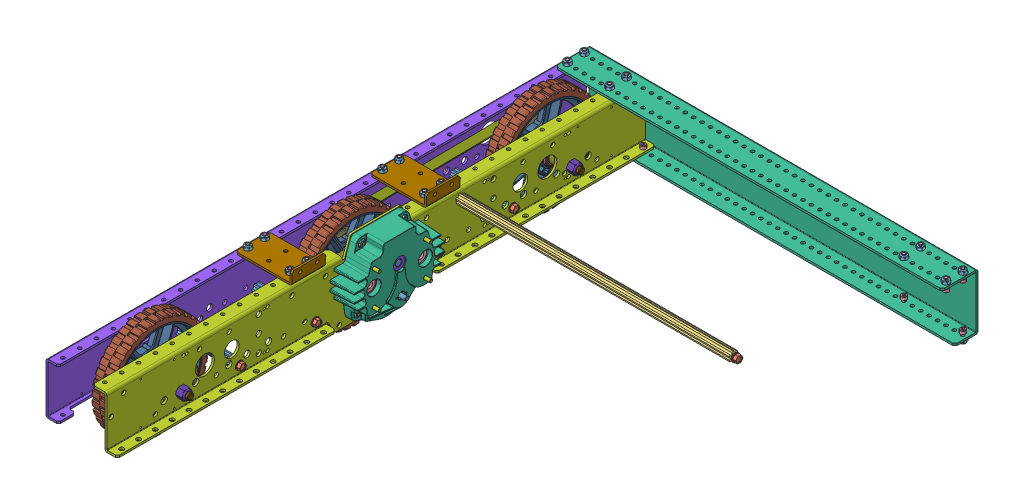
SolidWorks assembly AM14U3Long_Half, configuration Default. Lengths in mm.
Overall size (596.72 217.04 816.74).
154 component instances, 36 part files, 29 mates.
Components (placement in the parent):
- AM14U3Long_Frame_Half-1: AM14U3Long_Frame_Half [Default] at (0 136.144 -762.762) size (596.14 116.33 816.74)
  - 500Churro_3.375-1: 500Churro_3.375 [Default] at (-501.65 -66.929 448.437) x (0 0 1) z (-1 0 0) size (14.66 12.7 85.72)
  - 500Churro_3.375-2: 500Churro_3.375 [Default] at (-501.65 -66.929 562.737) x (0 0 1) z (-1 0 0) size (14.66 12.7 85.72)
  - 500Churro_3.375-3: 500Churro_3.375 [Default] at (-501.65 -66.929 264.287) x (0 0 1) z (-1 0 0) size (14.66 12.7 85.72)
  - 500Churro_3.375-4: 500Churro_3.375 [Default] at (-501.65 -66.929 149.987) x (0 0 1) z (-1 0 0) size (14.66 12.7 85.72)
  - ThreadRollingScrew_0.25-20x0.75-1: ThreadRollingScrew_0.25-20x0.75 [FHTS 0.25-20-G-0.75-C] at (-498.475 -66.929 562.737) x (-1 0 0) z (0 0.924225 0.381849) size (24.64 12.19 12.19)
  - ThreadRollingScrew_0.25-20x0.75-2: ThreadRollingScrew_0.25-20x0.75 [FHTS 0.25-20-G-0.75-C] at (-498.475 -66.929 448.437) x (-1 0 0) z (0 0.924225 0.381849) size (24.64 12.19 12.19)
  - ThreadRollingScrew_0.25-20x0.75-3: ThreadRollingScrew_0.25-20x0.75 [FHTS 0.25-20-G-0.75-C] at (-498.475 -66.929 264.287) x (-1 0 0) z (0 0.924225 0.381849) size (24.64 12.19 12.19)
  - ThreadRollingScrew_0.25-20x0.75-4: ThreadRollingScrew_0.25-20x0.75 [FHTS 0.25-20-G-0.75-C] at (-498.475 -66.929 149.987) x (-1 0 0) z (0 0.924225 0.381849) size (24.64 12.19 12.19)
  - ThreadRollingScrew_0.25-20x0.75-5: ThreadRollingScrew_0.25-20x0.75 [FHTS 0.25-20-G-0.75-C] at (-590.55 -66.929 562.737) size (24.64 12.19 12.19)
  - ThreadRollingScrew_0.25-20x0.75-6: ThreadRollingScrew_0.25-20x0.75 [FHTS 0.25-20-G-0.75-C] at (-590.55 -66.929 448.437) size (24.64 12.19 12.19)
  - ThreadRollingScrew_0.25-20x0.75-7: ThreadRollingScrew_0.25-20x0.75 [FHTS 0.25-20-G-0.75-C] at (-590.55 -66.929 149.987) size (24.64 12.19 12.19)
  - ThreadRollingScrew_0.25-20x0.75-8: ThreadRollingScrew_0.25-20x0.75 [FHTS 0.25-20-G-0.75-C] at (-590.55 -66.929 264.287) size (24.64 12.19 12.19)
  - ThreadRollingScrew_0.25-20x0.75-9: ThreadRollingScrew_0.25-20x0.75 [FHTS 0.25-20-G-0.75-C] at (-501.65 -15.494 229.362) size (24.64 12.19 12.19)
  - ThreadRollingScrew_0.25-20x0.75-10: ThreadRollingScrew_0.25-20x0.75 [FHTS 0.25-20-G-0.75-C] at (-82.55 -15.494 229.362) x (-1 0 0) z (0 -0.924225 -0.381849) size (24.64 12.19 12.19)
  - 500Churro_cut_16.25-1: 500Churro_cut_16.25 [Default] at (-85.725 -15.494 229.362) x (0 0.99241 0.122972) z (-1 0 0) size (14.66 12.7 412.75)
  - Screw_SHCS_10-32x0.5-27: Screw_SHCS_10-32x0.5 [HX-SHCS 0.19-32x1.375x1-C] at (-577.85 -11.43 -11.938) x (0 1 0) z (0 0 1) size (17.53 7.94 7.94)
  - Screw_SHCS_10-32x0.5-28: Screw_SHCS_10-32x0.5 [HX-SHCS 0.19-32x1.375x1-C] at (-577.85 -11.43 -37.338) x (0 1 0) z (0 0 1) size (17.53 7.94 7.94)
  - Screw_SHCS_10-32x0.5-29: Screw_SHCS_10-32x0.5 [HX-SHCS 0.19-32x1.375x1-C] at (-514.35 -11.43 -37.338) x (0 1 0) z (0 0 1) size (17.53 7.94 7.94)
  - Screw_SHCS_10-32x0.5-30: Screw_SHCS_10-32x0.5 [HX-SHCS 0.19-32x1.375x1-C] at (-514.35 -11.43 -11.938) x (0 1 0) z (0 0 1) size (17.53 7.94 7.94)
  - Screw_SHCS_10-32x0.5-31: Screw_SHCS_10-32x0.5 [HX-SHCS 0.19-32x1.375x1-C] at (-488.95 -73.152 -37.338) x (0 -1 0) z (0 0 1) size (17.53 7.94 7.94)
  - Screw_SHCS_10-32x0.5-32: Screw_SHCS_10-32x0.5 [HX-SHCS 0.19-32x1.375x1-C] at (-577.85 -73.152 -37.338) x (0 -1 0) z (0 0 1) size (17.53 7.94 7.94)
  - Screw_SHCS_10-32x0.5-40: Screw_SHCS_10-32x0.5 [HX-SHCS 0.19-32x1.375x1-C] at (-6.35 -11.176 -11.938) x (0 1 0) z (-0.991845 0 0.127447) size (17.53 7.94 7.94)
  - Screw_SHCS_10-32x0.5-41: Screw_SHCS_10-32x0.5 [HX-SHCS 0.19-32x1.375x1-C] at (-6.35 -11.176 -37.338) x (0 1 0) z (0.595464 0 0.803382) size (17.53 7.94 7.94)
  - Screw_SHCS_10-32x0.5-42: Screw_SHCS_10-32x0.5 [HX-SHCS 0.19-32x1.375x1-C] at (-69.85 -11.176 -11.938) x (0 1 0) z (0.578861 0 0.815426) size (17.53 7.94 7.94)
  - Screw_SHCS_10-32x0.5-43: Screw_SHCS_10-32x0.5 [HX-SHCS 0.19-32x1.375x1-C] at (-69.85 -11.176 -37.338) x (0 1 0) z (0.958905 0 0.283727) size (17.53 7.94 7.94)
  - Screw_SHCS_10-32x0.5-44: Screw_SHCS_10-32x0.5 [HX-SHCS 0.19-32x1.375x1-C] at (-6.35 -73.406 -37.338) x (0 -1 0) z (-0.989362 0 -0.145473) size (17.53 7.94 7.94)
  - Screw_SHCS_10-32x0.5-45: Screw_SHCS_10-32x0.5 [HX-SHCS 0.19-32x1.375x1-C] at (-95.25 -73.406 -37.338) x (0 -1 0) z (-0.875347 0 0.483496) size (17.53 7.94 7.94)
  - NylockNut_10-32-27: NylockNut_10-32 [Default] at (-69.85 0 -11.938) x (1 0 0) z (0 1 0) size (10.18 11.01 7.1)
  - NylockNut_10-32-28: NylockNut_10-32 [Default] at (-69.85 0 -37.338) x (1 0 0) z (0 1 0) size (10.18 11.01 7.1)
  - NylockNut_10-32-29: NylockNut_10-32 [Default] at (-6.35 0 -37.338) x (1 0 0) z (0 1 0) size (10.18 11.01 7.1)
  - NylockNut_10-32-30: NylockNut_10-32 [Default] at (-6.35 0 -11.938) x (1 0 0) z (0 1 0) size (10.18 11.01 7.1)
  - NylockNut_10-32-31: NylockNut_10-32 [Default] at (-6.35 -84.582 -37.338) x (1 0 0) z (0 -1 0) size (10.18 11.01 7.1)
  - NylockNut_10-32-32: NylockNut_10-32 [Default] at (-95.25 -84.582 -37.338) x (1 0 0) z (0 -1 0) size (10.18 11.01 7.1)
  - NylockNut_10-32-33: NylockNut_10-32 [Default] at (-514.35 0 -11.938) x (1 0 0) z (0 1 0) size (10.18 11.01 7.1)
  - NylockNut_10-32-34: NylockNut_10-32 [Default] at (-514.35 0 -37.338) x (1 0 0) z (0 1 0) size (10.18 11.01 7.1)
  - NylockNut_10-32-35: NylockNut_10-32 [Default] at (-577.85 0 -37.338) x (1 0 0) z (0 1 0) size (10.18 11.01 7.1)
  - NylockNut_10-32-36: NylockNut_10-32 [Default] at (-577.85 0 -11.938) x (1 0 0) z (0 1 0) size (10.18 11.01 7.1)
  - NylockNut_10-32-37: NylockNut_10-32 [Default] at (-488.95 -84.582 -37.338) x (1 0 0) z (0 -1 0) size (10.18 11.01 7.1)
  - NylockNut_10-32-38: NylockNut_10-32 [Default] at (-577.85 -84.582 -37.338) x (1 0 0) z (0 -1 0) size (10.18 11.01 7.1)
  - Screw_SHCS_10-32x0.5-46: Screw_SHCS_10-32x0.5 [HX-SHCS 0.19-32x1.375x1-C] at (-577.85 -11.43 445.262) x (0 1 0) z (0 0 1) size (17.53 7.94 7.94)
  - Screw_SHCS_10-32x0.5-47: Screw_SHCS_10-32x0.5 [HX-SHCS 0.19-32x1.375x1-C] at (-577.85 -11.43 470.662) x (0 1 0) z (0 0 1) size (17.53 7.94 7.94)
  - Screw_SHCS_10-32x0.5-48: Screw_SHCS_10-32x0.5 [HX-SHCS 0.19-32x1.375x1-C] at (-514.35 -11.43 445.262) x (0 1 0) z (0 0 1) size (17.53 7.94 7.94)
  - Screw_SHCS_10-32x0.5-49: Screw_SHCS_10-32x0.5 [HX-SHCS 0.19-32x1.375x1-C] at (-514.35 -11.43 470.662) x (0 1 0) z (0 0 1) size (17.53 7.94 7.94)
  - Screw_SHCS_10-32x0.5-50: Screw_SHCS_10-32x0.5 [HX-SHCS 0.19-32x1.375x1-C] at (-577.85 -11.43 267.462) x (0 1 0) z (0 0 1) size (17.53 7.94 7.94)
  - Screw_SHCS_10-32x0.5-51: Screw_SHCS_10-32x0.5 [HX-SHCS 0.19-32x1.375x1-C] at (-577.85 -11.43 242.062) x (0 1 0) z (0 0 1) size (17.53 7.94 7.94)
  - Screw_SHCS_10-32x0.5-52: Screw_SHCS_10-32x0.5 [HX-SHCS 0.19-32x1.375x1-C] at (-514.35 -11.43 242.062) x (0 1 0) z (0 0 1) size (17.53 7.94 7.94)
  - Screw_SHCS_10-32x0.5-53: Screw_SHCS_10-32x0.5 [HX-SHCS 0.19-32x1.375x1-C] at (-514.35 -11.43 267.462) x (0 1 0) z (0 0 1) size (17.53 7.94 7.94)
  - NylockNut_10-32-39: NylockNut_10-32 [Default] at (-514.35 -0.254 267.462) x (1 0 0) z (0 1 0) size (10.18 11.01 7.1)
  - NylockNut_10-32-40: NylockNut_10-32 [Default] at (-514.35 -0.254 242.062) x (1 0 0) z (0 1 0) size (10.18 11.01 7.1)
  - NylockNut_10-32-41: NylockNut_10-32 [Default] at (-577.85 -0.254 267.462) x (1 0 0) z (0 1 0) size (10.18 11.01 7.1)
  - NylockNut_10-32-42: NylockNut_10-32 [Default] at (-577.85 -0.254 242.062) x (1 0 0) z (0 1 0) size (10.18 11.01 7.1)
  - NylockNut_10-32-43: NylockNut_10-32 [Default] at (-514.35 -0.254 470.662) x (1 0 0) z (0 1 0) size (10.18 11.01 7.1)
  - NylockNut_10-32-44: NylockNut_10-32 [Default] at (-577.85 -0.254 470.662) x (1 0 0) z (0 1 0) size (10.18 11.01 7.1)
  - NylockNut_10-32-45: NylockNut_10-32 [Default] at (-577.85 -0.254 445.262) x (1 0 0) z (0 1 0) size (10.18 11.01 7.1)
  - NylockNut_10-32-46: NylockNut_10-32 [Default] at (-514.35 -0.254 445.262) x (1 0 0) z (0 1 0) size (10.18 11.01 7.1)
  - AM14U3EndPlate_Long-1: AM14U3EndPlate_Long [Default] at (-488.098 60.9785 -76.8664) x (1 0 0) z (0 -1 0) size (584.2 53.97 84.58)
  - AM14U3InnerPlate_Long-1: AM14U3InnerPlate_Long [Default] at (-501.65 -77.216 762.762) x (0 0 -1) z (0 -1 0) size (812.8 38.1 116.33)
  - AM14U3OuterPlate_Long-1: AM14U3OuterPlate_Long [DefaultSM-FLAT-PATTERN] at (-587.375 -77.216 -50.038) x (0 0 1) z (0 -1 0) size (812.8 19.05 77.72)
  - Bracket_2x3-1: Bracket_2x3 [Default] at (-584.2 -3.429 496.062) size (85.72 19.05 50.8)
  - Bracket_2x3-2: Bracket_2x3 [Default] at (-584.2 -3.429 292.862) size (85.72 19.05 50.8)
- Wheel-6inHiGrip_Outer-1: Wheel-6inHiGrip_Outer [Default] at (-576.1365 22.5372 -253.3218) x (1 0 0) z (0 -0.142471 0.989799) size (85.56 191.55 191.55)
  - Wheel_6inHiGrip-1: Wheel_6inHiGrip [Default] at (83.7987 67.439 110.9939) size (35.05 191.55 191.55)
    - Wheel_6inHiGrip_Wheel-1: Wheel_6inHiGrip_Wheel [Default] at (-52.6446 9.4231 21.378) size (35.05 132.08 132.08)
    - Wheel_6inHiGrip_Tread-1: Wheel_6inHiGrip_Tread [Default] at (-65.3446 9.4231 21.378) x (0 -0.304368 -0.952555) z (1 0 0) size (152.4 152.4 25.58)
  - HalfPulley_42t5mm-1: HalfPulley_42t5mm [Default] at (47.6006 76.862 132.3719) x (1 0 0) z (0 -0.5 0.866025) size (13 74.23 74.23)
  - HalfPulley_42t5mm-2: HalfPulley_42t5mm [Default] at (64.263 76.862 132.3719) x (-1 0 0) z (0 -0.499927 0.866067) size (13 74.23 74.23)
  - Bearing_1614ZZ-1: Bearing_1614ZZ [Default] at (62.612 76.862 132.3719) x (0 -0.157148 -0.987575) z (-1 0 0) size (28.57 28.57 9.53)
  - Bearing_1614ZZ-2: Bearing_1614ZZ [Default] at (15.2791 76.862 132.3719) x (0 0 -1) z (1 0 0) size (28.57 28.57 9.53)
  - ThreadFormingScrew_10-24x1.25-1: ThreadFormingScrew_10-24x1.25 [93882A213] at (63.247 76.8605 108.5602) x (0 0 -1) z (1 0 0) size (10.52 10.52 35.59)
  - ThreadFormingScrew_10-24x1.25-2: ThreadFormingScrew_10-24x1.25 [93882A213] at (63.247 97.4833 120.4656) x (0 0 -1) z (1 0 0) size (10.52 10.52 35.59)
  - ThreadFormingScrew_10-24x1.25-3: ThreadFormingScrew_10-24x1.25 [93882A213] at (63.247 56.2398 144.2799) x (0 0 -1) z (1 0 0) size (10.52 10.52 35.59)
  - ThreadFormingScrew_10-24x1.25-4: ThreadFormingScrew_10-24x1.25 [93882A213] at (63.247 76.8625 156.1852) x (0 -0.95788 -0.287168) z (1 0 0) size (10.52 10.52 35.59)
  - ThreadFormingScrew_10-24x1.25-5: ThreadFormingScrew_10-24x1.25 [93882A213] at (63.247 97.4843 144.2781) x (0 -0.868976 0.494854) z (1 0 0) size (10.52 10.52 35.59)
  - ThreadFormingScrew_10-24x1.25-6: ThreadFormingScrew_10-24x1.25 [93882A213] at (63.247 56.2388 120.4674) x (0 -0.977348 -0.211637) z (1 0 0) size (10.52 10.52 35.59)
  - Spacer_0.28x0.382-1: Spacer_0.28x0.382 [Default] at (74.4865 76.862 132.3719) x (0 -0.35357 0.935408) z (-1 0 0) size (13.16 13.16 7.11)
  - Spacer_0.85x0.38-1: Spacer_0.85x0.38 [Default] at (-11.0734 76.862 132.3719) x (0 0 -1) z (1 0 0) size (19.05 19.05 21.59)
- Wheel-6inHiGrip_Outer-2: Wheel-6inHiGrip_Outer [Default] at (-512.7234 228.3276 -664.619) x (-1 0 0) z (0 -0.960203 0.279302) size (85.56 191.55 191.55)
  - Wheel_6inHiGrip-1: Wheel_6inHiGrip [Default] at (83.7987 67.439 110.9939) size (35.05 191.55 191.55)
    - Wheel_6inHiGrip_Wheel-1: Wheel_6inHiGrip_Wheel [Default] at (-52.6446 9.4231 21.378) size (35.05 132.08 132.08)
    - Wheel_6inHiGrip_Tread-1: Wheel_6inHiGrip_Tread [Default] at (-65.3446 9.4231 21.378) x (0 -0.304368 -0.952555) z (1 0 0) size (152.4 152.4 25.58)
  - HalfPulley_42t5mm-1: HalfPulley_42t5mm [Default] at (47.6006 76.862 132.3719) x (1 0 0) z (0 -0.5 0.866025) size (13 74.23 74.23)
  - HalfPulley_42t5mm-2: HalfPulley_42t5mm [Default] at (64.263 76.862 132.3719) x (-1 0 0) z (0 -0.499927 0.866067) size (13 74.23 74.23)
  - Bearing_1614ZZ-1: Bearing_1614ZZ [Default] at (62.612 76.862 132.3719) x (0 -0.157148 -0.987575) z (-1 0 0) size (28.57 28.57 9.53)
  - Bearing_1614ZZ-2: Bearing_1614ZZ [Default] at (15.2791 76.862 132.3719) x (0 0 -1) z (1 0 0) size (28.57 28.57 9.53)
  - ThreadFormingScrew_10-24x1.25-1: ThreadFormingScrew_10-24x1.25 [93882A213] at (63.247 76.8605 108.5602) x (0 0 -1) z (1 0 0) size (10.52 10.52 35.59)
  - ThreadFormingScrew_10-24x1.25-2: ThreadFormingScrew_10-24x1.25 [93882A213] at (63.247 97.4833 120.4656) x (0 0 -1) z (1 0 0) size (10.52 10.52 35.59)
  - ThreadFormingScrew_10-24x1.25-3: ThreadFormingScrew_10-24x1.25 [93882A213] at (63.247 56.2398 144.2799) x (0 0 -1) z (1 0 0) size (10.52 10.52 35.59)
  - ThreadFormingScrew_10-24x1.25-4: ThreadFormingScrew_10-24x1.25 [93882A213] at (63.247 76.8625 156.1852) x (0 -0.95788 -0.287168) z (1 0 0) size (10.52 10.52 35.59)
  - ThreadFormingScrew_10-24x1.25-5: ThreadFormingScrew_10-24x1.25 [93882A213] at (63.247 97.4843 144.2781) x (0 -0.868976 0.494854) z (1 0 0) size (10.52 10.52 35.59)
  - ThreadFormingScrew_10-24x1.25-6: ThreadFormingScrew_10-24x1.25 [93882A213] at (63.247 56.2388 120.4674) x (0 -0.977348 -0.211637) z (1 0 0) size (10.52 10.52 35.59)
  - Spacer_0.28x0.382-1: Spacer_0.28x0.382 [Default] at (74.4865 76.862 132.3719) x (0 -0.35357 0.935408) z (-1 0 0) size (13.16 13.16 7.11)
  - Spacer_0.85x0.38-1: Spacer_0.85x0.38 [Default] at (-11.0734 76.862 132.3719) x (0 0 -1) z (1 0 0) size (19.05 19.05 21.59)
- Wheel_6inHiGrip_Center-1: Wheel_6inHiGrip_Center [Default] at (-512.6497 0.0121 -273.639) x (-1 0 0) z (0 -0.005085 -0.999987) size (81.42 191.55 191.55)
  - Wheel_6inHiGrip-1: Wheel_6inHiGrip [Default] at (83.7987 67.439 110.9939) size (35.05 191.55 191.55)
    - Wheel_6inHiGrip_Wheel-1: Wheel_6inHiGrip_Wheel [Default] at (-52.6446 9.4231 21.378) size (35.05 132.08 132.08)
    - Wheel_6inHiGrip_Tread-1: Wheel_6inHiGrip_Tread [Default] at (-65.3446 9.4231 21.378) x (0 -0.304368 -0.952555) z (1 0 0) size (152.4 152.4 25.58)
  - HalfPulley_42t5mm-1: HalfPulley_42t5mm [Default] at (47.6006 76.862 132.3719) x (1 0 0) z (0 -0.5 0.866025) size (13 74.23 74.23)
  - HalfPulley_42t5mm-2: HalfPulley_42t5mm [Default] at (64.263 76.862 132.3719) x (-1 0 0) z (0 -0.499927 0.866067) size (13 74.23 74.23)
  - ThreadFormingScrew_10-24x1.25-1: ThreadFormingScrew_10-24x1.25 [93882A213] at (63.247 76.8605 108.5602) x (0 0 -1) z (1 0 0) size (10.52 10.52 35.59)
  - ThreadFormingScrew_10-24x1.25-2: ThreadFormingScrew_10-24x1.25 [93882A213] at (63.247 97.4833 120.4656) x (0 0 -1) z (1 0 0) size (10.52 10.52 35.59)
  - ThreadFormingScrew_10-24x1.25-3: ThreadFormingScrew_10-24x1.25 [93882A213] at (63.247 56.2398 144.2799) x (0 0 -1) z (1 0 0) size (10.52 10.52 35.59)
  - ThreadFormingScrew_10-24x1.25-4: ThreadFormingScrew_10-24x1.25 [93882A213] at (63.247 76.8625 156.1852) x (0 -0.95788 -0.287168) z (1 0 0) size (10.52 10.52 35.59)
  - ThreadFormingScrew_10-24x1.25-5: ThreadFormingScrew_10-24x1.25 [93882A213] at (63.247 97.4843 144.2781) x (0 -0.868976 0.494854) z (1 0 0) size (10.52 10.52 35.59)
  - ThreadFormingScrew_10-24x1.25-6: ThreadFormingScrew_10-24x1.25 [93882A213] at (63.247 56.2388 120.4674) x (0 -0.748729 -0.662876) z (1 0 0) size (10.52 10.52 35.59)
  - HalfPulley_42t5mm-3: HalfPulley_42t5mm [Default] at (-1.9548 76.8628 132.3714) x (1 0 0) z (0 -1 -0.000063) size (13 74.23 74.23)
  - HalfPulley_42t5mm-4: HalfPulley_42t5mm [Default] at (14.7076 76.8628 132.3714) x (-1 0 0) z (0 -1 0.000021) size (13 74.23 74.23)
  - HexHub_500EX-1: HexHub_500EX [Default] at (-8.3048 76.8628 132.3714) x (0 -0.866025 -0.5) z (0 -0.5 0.866025) size (55.37 25.4 51.33)
  - ThreadFormingScrew_10-24x1.25-7: ThreadFormingScrew_10-24x1.25 [93882A213] at (-5.2568 97.485 120.4652) x (0 0 1) z (-1 0 0) size (10.52 10.52 35.59)
  - ThreadFormingScrew_10-24x1.25-8: ThreadFormingScrew_10-24x1.25 [93882A213] at (-5.2568 76.8628 108.5589) x (0 0 1) z (-1 0 0) size (10.52 10.52 35.59)
  - ThreadFormingScrew_10-24x1.25-9: ThreadFormingScrew_10-24x1.25 [93882A213] at (-5.2568 56.2406 120.4652) x (0 0 1) z (-1 0 0) size (10.52 10.52 35.59)
  - ThreadFormingScrew_10-24x1.25-10: ThreadFormingScrew_10-24x1.25 [93882A213] at (-5.2568 97.485 144.2777) x (0 -0.99374 -0.111715) z (-1 0 0) size (10.52 10.52 35.59)
  - ThreadFormingScrew_10-24x1.25-11: ThreadFormingScrew_10-24x1.25 [93882A213] at (-5.2568 56.2406 144.2777) x (0 -0.138911 0.990305) z (-1 0 0) size (10.52 10.52 35.59)
  - ThreadFormingScrew_10-24x1.25-12: ThreadFormingScrew_10-24x1.25 [93882A213] at (-5.2568 76.8628 156.1839) x (0 -0.98811 -0.15375) z (-1 0 0) size (10.52 10.52 35.59)
  - Spacer_Hex_0.57x0.5-1: Spacer_Hex_0.57x0.5 [Default] at (57.8495 76.862 132.3719) x (0 -0.866025 -0.5) z (0 -0.5 0.866025) size (28.55 14.48 28.55)
- ToughboxMini-1: ToughboxMini [Default] at (-549.0167 66.1299 -315.2992) x (0 0.001296 0.999999) z (-1 0 0) size (140.05 123.17 142.29) (flexible)
  - TBMiniSmallHexShaft-1: TBMiniSmallHexShaft [Default] at (-128.7801 70.693 -52.3959) x (-0.996714 0.081004 0) z (0.081004 0.996714 0) size (11 38.23 9.52)
  - ToughboxLargeClusterGear_Hex_50t0.375-1: ToughboxLargeClusterGear_Hex_50t0.375 [Default] at (-91.0349 50.9043 -67.5597) x (-0.996714 0.081004 0) z (0 0 -1) size (65.97 66.04 10.16)
  - Bearing_FR6ZZ-1: Bearing_FR6ZZ [Default] at (-96.247 60.278 -52.5991) x (-0.893862 0.448342 0) z (0 0 1) size (24.69 24.69 7.16)
  - NylockNut_10-32-1: NylockNut_10-32 [Default] at (-129.8464 -8.0737 -56.3837) x (0.501678 0.865055 0) z (0 0 -1) size (10.18 11.01 7.1)
  - NylockNut_10-32-2: NylockNut_10-32 [Default] at (-59.2462 80.7349 -56.3837) x (0.999999 -0.001296 0) z (0 0 -1) size (10.18 11.01 7.1)
  - NylockNut_10-32-3: NylockNut_10-32 [Default] at (-122.7461 80.8172 -56.3837) x (0.500567 0.865698 0) z (0 0 -1) size (10.18 11.01 7.1)
  - NylockNut_10-32-4: NylockNut_10-32 [Default] at (-52.3764 -8.1741 -56.3837) x (-0.501678 -0.865055 0) z (0 0 -1) size (10.18 11.01 7.1)
  - Washer_5-16-1: Washer_5-16 [Default] at (-52.3162 38.3079 -77.7705) x (0.171117 0.985251 0) z (0 0 -1) size (17.53 17.53 1.47)
  - Washer_5-16-2: Washer_5-16 [Default] at (-52.3162 38.3079 -76.2973) x (0.897267 -0.441488 0) z (0 0 -1) size (17.53 17.53 1.47)
  - Washer_5-16-3: Washer_5-16 [Default] at (-129.7861 38.4083 -77.7705) x (-0.990116 0.140253 0) z (0 0 1) size (17.53 17.53 1.47)
  - Washer_5-16-4: Washer_5-16 [Default] at (-129.7861 38.4083 -79.2437) x (-0.681761 0.731575 0) z (0 0 1) size (17.53 17.53 1.47)
  - CIMGear_14t8mm-1: CIMGear_14t8mm [Default] at (-52.3162 38.3079 -63.5973) x (0.912005 0.410178 0) z (0 0 -1) size (20.03 20.32 12.7)
  - CIMGear_14t8mm-2: CIMGear_14t8mm [Default] at (-129.7861 38.4083 -63.5973) x (0.952996 -0.302983 0) z (0 0 -1) size (20.03 20.32 12.7)
  - TBMiniHousing-1: TBMiniHousing [Default] at (-91.0876 10.1882 -86.3557) x (0.999999 -0.001296 0) z (0 0 1) size (139.9 118.55 41.54)
  - Screw_SHCS_10-32x0.625-1: Screw_SHCS_10-32x0.625 [Default] at (-52.2832 63.7078 -74.4685) x (-0.564778 -0.825243 0) z (-0.825243 0.564778 0) size (7.82 20.65 7.82)
  - Screw_SHCS_10-32x0.625-2: Screw_SHCS_10-32x0.625 [Default] at (-122.7461 80.8172 -42.5915) x (0.507484 -0.861661 0) z (-0.861661 -0.507484 0) size (7.82 20.65 7.82)
  - Screw_SHCS_10-32x0.625-3: Screw_SHCS_10-32x0.625 [Default] at (-52.3764 -8.1741 -42.5915) x (0.507484 -0.861661 0) z (-0.861661 -0.507484 0) size (7.82 20.65 7.82)
  - Screw_SHCS_10-32x0.625-4: Screw_SHCS_10-32x0.625 [Default] at (-129.8464 -8.0737 -42.5915) x (0.507484 -0.861661 0) z (-0.861661 -0.507484 0) size (7.82 20.65 7.82)
  - Screw_SHCS_10-32x0.625-5: Screw_SHCS_10-32x0.625 [Default] at (-59.2462 80.7349 -42.5915) x (0.740711 -0.671824 0) z (-0.671824 -0.740711 0) size (7.82 20.65 7.82)
  - Screw_SHCS_10-32x0.625-6: Screw_SHCS_10-32x0.625 [Default] at (-52.3491 12.9079 -74.4685) x (-0.564778 -0.825243 0) z (-0.825243 0.564778 0) size (7.82 20.65 7.82)
  - Screw_SHCS_10-32x0.625-7: Screw_SHCS_10-32x0.625 [Default] at (-129.7532 63.8083 -74.4685) x (-0.966277 -0.257503 0) z (-0.257503 0.966277 0) size (7.82 20.65 7.82)
  - Screw_SHCS_10-32x0.625-8: Screw_SHCS_10-32x0.625 [Default] at (-129.819 13.0083 -74.4685) x (-0.99652 0.083357 0) z (0.083357 0.99652 0) size (7.82 20.65 7.82)
  - Bearing_R6ZZ-3: Bearing_R6ZZ [Default] at (-91.0349 50.9043 -84.8317) x (0.958138 -0.286306 0) z (0 0 1) size (22.23 22.23 7.11)
  - Bearing_R6ZZ-4: Bearing_R6ZZ [Default] at (-91.0876 10.1882 -84.8317) x (-0.661529 0.74992 0) z (0 0 1) size (22.23 22.23 7.11)
  - RetainingClip-1: RetainingClip [Default] at (-129.7861 38.4083 -63.5973) x (0 0 1) z (-1 0 0) size (1.09 14.83 14.83)
  - RetainingClip-2: RetainingClip [Default] at (-52.3162 38.3079 -63.5973) x (0 0 1) z (-1 0 0) size (1.09 14.83 14.83)
  - ExternalKlipring-1: ExternalKlipring [Default] at (-91.0876 10.1882 -64.4355) x (0.996411 -0.084651 0) z (0 0 1) size (19.07 20.96 1.27)
  - HexBearing_FR8ZZ-1: HexBearing_FR8ZZ [Default] at (-91.0876 10.1882 -44.6717) x (-0.999993 -0.003789 0) z (0 0 -1) size (31.12 31.12 7.93)
  - SmallClusterGear_Hex_16t0.375-1: SmallClusterGear_Hex_16t0.375 [Default] at (-91.0349 50.9043 -67.5597) x (0 0 1) z (-0.568509 -0.822677 0) size (15.19 22.57 22.57)
  - LargeOutputGear_Hex_48t0.5-1: LargeOutputGear_Hex_48t0.5 [Default] at (-91.0876 10.1882 -63.1655) x (0 0 1) z (0.503278 -0.864125 0) size (10.21 63.42 63.42)
  - TBMiniHexOutputShaft-2: TBMiniHexOutputShaft [Default] at (-129.4577 26.7119 -52.3197) x (-0.999993 -0.003789 0) z (-0.003789 0.999993 0) size (14.66 142.29 12.7)
- Bearing_Hex_FR8ZZ-1: Bearing_Hex_FR8ZZ [Default] at (-593.7783 76.2 -406.4) x (0 0.868557 0.49559) z (1 0 0) size (31.12 31.12 7.93)
- Belt_15mm_Long-1: Belt_15mm_Long [Default] at (-511.8735 79.756 -111.3496) x (0 -0.012051 -0.999927) z (0 0.999927 -0.012051) size (368.15 15 73.08)
- Belt_15mm_Long-2: Belt_15mm_Long [Default] at (-576.9127 76.2 -406.4) x (0 0.012051 -0.999927) z (0 -0.999927 -0.012051) size (368.15 15 73.08)
- NylockNut_0.375-16-1: NylockNut_0.375-16 [91831A127] at (-498.475 79.7563 -701.4504) x (0 -1 0) z (0 0 1) size (14.29 12 16.5)
- NylockNut_0.375-16-2: NylockNut_0.375-16 [91831A127] at (-498.475 79.7563 -111.3496) x (0 -1 0) z (0 0 1) size (14.29 12 16.5)
- HHSBolt_0.375-16x4.25-1: HHSBolt_0.375-16x4.25 [HFBOLT 0.375-16x2.5x1-C] at (-596.7222 79.756 -111.3496) size (114.12 16.48 14.27)
- HHSBolt_0.375-16x4.25-2: HHSBolt_0.375-16x4.25 [HFBOLT 0.375-16x2.5x1-C] at (-596.7222 79.756 -701.4504) size (114.12 16.48 14.27)
Mates (geometry in assembly coordinates):
- Concentric1: concentric aligned: cylinder of AM14U3Long_Frame_Half-1/AM14U3InnerPlate_Long-1 through (-520.7 79.756 -111.3496) axis (1 0 0) radius 4.826; cylinder of Wheel-6inHiGrip_Outer-1/Spacer_0.28x0.382-1 through (-508.762 79.756 -111.3496) axis (1 0 0) radius 6.5786
- Coincident1: coincident anti-aligned: plane of AM14U3Long_Frame_Half-1/AM14U3InnerPlate_Long-1 through (-501.65 128.778 0) normal (-1 0 0); plane of Wheel-6inHiGrip_Outer-1/Spacer_0.28x0.382-1 through (-501.65 79.756 -111.3496) normal (1 0 0)
- Concentric2: concentric anti-aligned: cylinder of AM14U3Long_Frame_Half-1/AM14U3InnerPlate_Long-1 through (-520.7 79.756 -701.4504) axis (1 0 0) radius 4.826; cylinder of Wheel-6inHiGrip_Outer-2/Spacer_0.28x0.382-1 through (-580.0979 79.756 -701.4504) axis (-1 0 0) radius 6.5786
- Coincident2: coincident anti-aligned: plane of AM14U3Long_Frame_Half-1/AM14U3InnerPlate_Long-1 through (-501.65 128.778 0) normal (-1 0 0); plane of Wheel-6inHiGrip_Outer-2/Spacer_0.85x0.38-1 through (-501.65 79.756 -701.4504) normal (1 0 0)
- Concentric3: concentric anti-aligned: cylinder of AM14U3Long_Frame_Half-1/AM14U3InnerPlate_Long-1 through (-501.65 76.2 -406.4) axis (1 0 0) radius 14.2875; cylinder of ToughboxMini-1/HexBearing_FR8ZZ-1 through (-496.4176 76.2 -406.4) axis (-1 0 0) radius 14.2875
- Parallel1: parallel: plane of AM14U3Long_Frame_Half-1/AM14U3InnerPlate_Long-1 through (-498.475 156.21 -454.025) normal (0 1 0); line of ToughboxMini-1/TBMiniHousing-1 through (-497.9493 155.7672 -438.15) axis (0 0 1)
- Coincident4: coincident anti-aligned: plane of AM14U3Long_Frame_Half-1/AM14U3InnerPlate_Long-1 through (-498.475 128.778 0) normal (1 0 0); plane of ToughboxMini-1/TBMiniHousing-1 through (-498.475 76.2 -406.4) normal (-1 0 0)
- Concentric41: concentric aligned: cylinder of AM14U3Long_Frame_Half-1/AM14U3OuterPlate_Long-1 through (-587.375 76.2 -406.4) axis (-1 0 0) radius 14.2875; cylinder of Bearing_Hex_FR8ZZ-1 through (-585.851 76.2 -406.4) axis (-1 0 0) radius 13.97
- Coincident51: coincident anti-aligned: plane of AM14U3Long_Frame_Half-1/AM14U3OuterPlate_Long-1 through (-587.375 128.778 -812.8) normal (1 0 0); plane of Bearing_Hex_FR8ZZ-1 through (-587.375 88.3337 -399.4766) normal (-1 0 0)
- Coincident6: coincident anti-aligned: plane of ToughboxMini-1/TBMiniHexOutputShaft-2 through (-471.297 76.2373 -399.0677) normal (0 0.504397 0.863472); plane of Bearing_Hex_FR8ZZ-1 through (-585.851 76.2373 -399.0677) normal (0 -0.504397 -0.863472)
- Concentric5: concentric aligned: cylinder of Wheel_6inHiGrip_Center-1/HexHub_500EX-1 through (-478.2153 76.2008 -406.3996) axis (-1 0 0) radius 9.2382; cylinder of ToughboxMini-1/HexBearing_FR8ZZ-1 through (-496.4176 76.2 -406.4) axis (-1 0 0) radius 14.2875
- Parallel2: parallel aligned: plane of Wheel_6inHiGrip_Center-1/HexHub_500EX-1 through (-504.3449 82.5447 -410.1054) normal (0 -0.49559 0.868557); plane of ToughboxMini-1/TBMiniHexOutputShaft-2 through (-471.297 69.8687 -402.7016) normal (0 -0.49559 0.868557)
- Coincident8: coincident anti-aligned: plane of Wheel_6inHiGrip_Center-1/HexHub_500EX-1 through (-504.3449 76.2008 -406.3996) normal (1 0 0); plane of ToughboxMini-1/HexBearing_FR8ZZ-1 through (-504.3449 76.2 -406.4) normal (-1 0 0)
- Concentric6: concentric anti-aligned: cylinder of Wheel-6inHiGrip_Outer-1/Spacer_0.85x0.38-1 through (-565.6199 79.756 -111.3496) axis (-1 0 0) radius 9.525; cylinder of Belt_15mm_Long-1 through (-526.8735 79.756 -111.3496) axis (1 0 0) radius 35.0139
- Concentric7: concentric anti-aligned: cylinder of Bearing_Hex_FR8ZZ-1 through (-585.851 76.2 -406.4) axis (-1 0 0) radius 14.2875; cylinder of Belt_15mm_Long-1 through (-526.8735 76.2 -406.4) axis (1 0 0) radius 35.0139
- Coincident9: coincident anti-aligned: plane of Wheel-6inHiGrip_Outer-1/HalfPulley_42t5mm-2 through (-511.8735 79.756 -111.3496) normal (-1 0 0); plane of Belt_15mm_Long-1 through (-511.8735 79.756 -111.3496) normal (1 0 0)
- Concentric8: concentric anti-aligned: cylinder of Wheel-6inHiGrip_Outer-2/Spacer_0.85x0.38-1 through (-523.24 79.756 -701.4504) axis (1 0 0) radius 9.525; cylinder of Belt_15mm_Long-2 through (-561.9127 79.756 -701.4504) axis (-1 0 0) radius 35.0139
- Concentric9: concentric anti-aligned: cylinder of Bearing_Hex_FR8ZZ-1 through (-585.851 76.2 -406.4) axis (-1 0 0) radius 14.2875; circle of Belt_15mm_Long-2
- Coincident10: coincident anti-aligned: plane of Wheel_6inHiGrip_Center-1/HalfPulley_42t5mm-2 through (-576.9127 76.2 -406.4) normal (1 0 0); plane of Belt_15mm_Long-2 through (-576.9127 76.2 -406.4) normal (-1 0 0)
- Coincident13: coincident anti-aligned: plane of AM14U3Long_Frame_Half-1/AM14U3InnerPlate_Long-1 through (-498.475 128.778 0) normal (1 0 0); plane of NylockNut_0.375-16-2 through (-498.475 86.9 -123.723) normal (-1 0 0)
- Coincident14: coincident anti-aligned: plane of AM14U3Long_Frame_Half-1/AM14U3InnerPlate_Long-1 through (-498.475 128.778 0) normal (1 0 0); plane of NylockNut_0.375-16-1 through (-498.475 86.9 -713.8237) normal (-1 0 0)
- Coincident125: coincident aligned: plane of AM14U3Long_Frame_Half-1/AM14U3InnerPlate_Long-1 through (-501.65 132.715 0) normal (0 0 1); plane of assembly through (0 0 0) normal (0 0 1)
- Coincident126: coincident aligned: plane of AM14U3Long_Frame_Half-1/AM14U3EndPlate_Long-1 through (0 54.737 -813.562) normal (1 0 0); plane of assembly through (0 0 0) normal (1 0 0)
- Parallel3: parallel anti-aligned: plane of AM14U3Long_Frame_Half-1/AM14U3InnerPlate_Long-1 through (-498.475 54.991 -812.8) normal (0 -1 0); plane of assembly through (0 0 0) normal (0 1 0)
- Tangent1: tangent: circle of Wheel_6inHiGrip_Center-1/Wheel_6inHiGrip-1/Wheel_6inHiGrip_Tread-1; plane of assembly through (0 0 0) normal (0 1 0)
- Concentric112: concentric aligned: cylinder of AM14U3Long_Frame_Half-1/AM14U3OuterPlate_Long-1 through (-479.424 79.756 -111.3496) axis (-1 0 0) radius 4.826; cylinder of HHSBolt_0.375-16x4.25-1 through (-596.7222 79.756 -111.3496) axis (-1 0 0) radius 4.7625
- Coincident127: coincident anti-aligned: plane of AM14U3Long_Frame_Half-1/AM14U3OuterPlate_Long-1 through (-590.55 128.778 -812.8) normal (-1 0 0); plane of HHSBolt_0.375-16x4.25-1 through (-590.55 87.9976 -111.3496) normal (1 0 0)
- Concentric1131: concentric aligned: cylinder of AM14U3Long_Frame_Half-1/AM14U3OuterPlate_Long-1 through (-479.424 79.756 -701.4504) axis (-1 0 0) radius 4.826; cylinder of HHSBolt_0.375-16x4.25-2 through (-596.7222 79.756 -701.4504) axis (-1 0 0) radius 7.1374
- Coincident1281: coincident anti-aligned: plane of AM14U3Long_Frame_Half-1/AM14U3OuterPlate_Long-1 through (-590.55 128.778 -812.8) normal (-1 0 0); plane of HHSBolt_0.375-16x4.25-2 through (-590.55 87.9976 -701.4504) normal (1 0 0)
